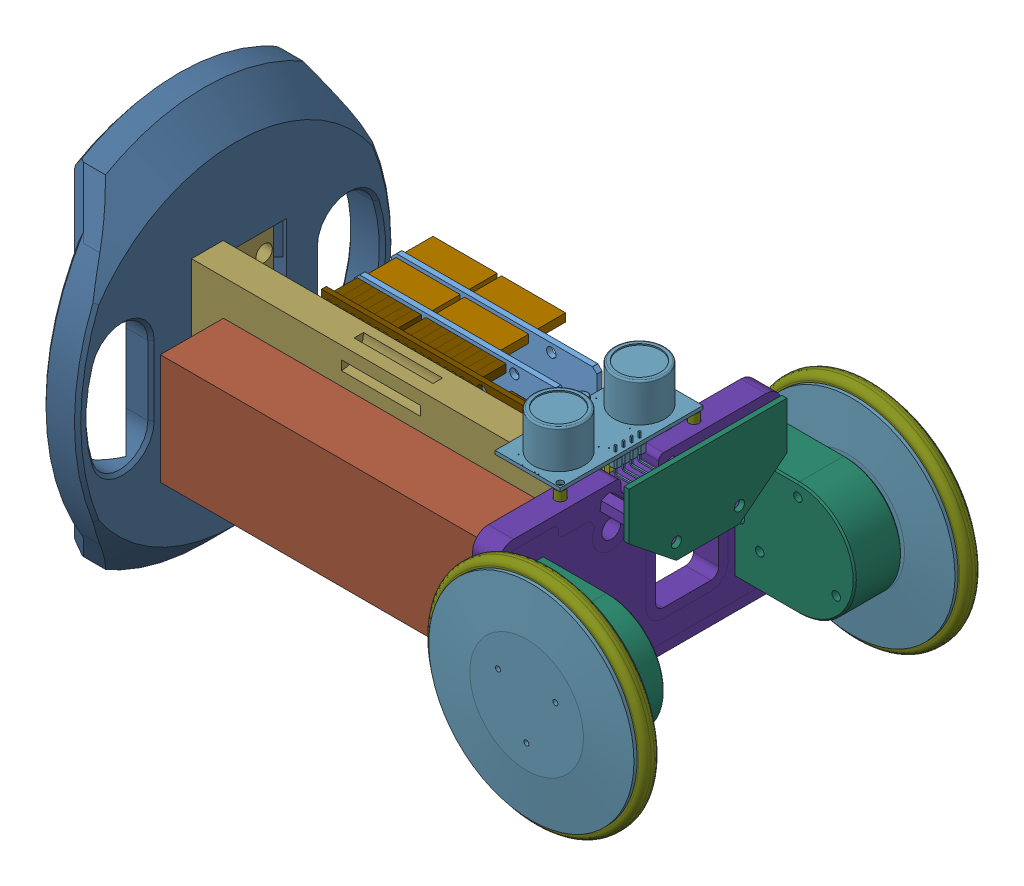
SolidWorks assembly blanceCar-BLDC-双轮平衡平台-立式, configuration 默认. Lengths in mm.
Overall size (212.5 125 111.7).
233 component instances, 36 part files, 54 mates.
Components (placement in the parent):
- BLDC一体驱动-typeA-1: BLDC一体驱动-typeA [默认] at (10.5873 0 95.3779) size (88.95 88.95 25.75)
  - lgt328-simpleFoc-drv8313.step-1: lgt328-simpleFoc-drv8313.step [默认] at origin size (28.6 30.99 10.29)
    - LQFP-32_7x7mm_P0.8mm.step-1: LQFP-32_7x7mm_P0.8mm.step [默认] at (5.381 2.9 1.65) size (9 9 1.5)
      - SOLID.step-1: SOLID.step [默认] at origin size (9 9 1.5)
    - C_0603_1608Metric.step-1: C_0603_1608Metric.step [默认] at (-3.2065 2.01 1.65) x (-1 0 0) z (0 0 1) size (1.6 0.8 0.8)
      - SOLID-0.step-1: SOLID-0.step [默认] at origin size (1.6 0.8 0.8)
    - C_0603_1608Metric.step-2: C_0603_1608Metric.step [默认] at (-3.2165 3.53 1.65) x (-1 0 0) z (0 0 1) size (1.6 0.8 0.8)
      - SOLID-0.step-1: SOLID-0.step [默认] at origin size (1.6 0.8 0.8)
    - C_0603_1608Metric.step-3: C_0603_1608Metric.step [默认] at (0.3835 7.85 1.65) x (-1 0 0) z (0 0 1) size (1.6 0.8 0.8)
      - SOLID-0.step-1: SOLID-0.step [默认] at origin size (1.6 0.8 0.8)
    - SW_SPST_B3U-1000P.step-1: SW_SPST_B3U-1000P.step [默认] at (5.7412 10.211 1.65) size (4 2.51 1.59)
      - SOLID-1.step-1: SOLID-1.step [默认] at origin size (4 2.51 1.59)
    - R_0603_1608Metric.step-1: R_0603_1608Metric.step [默认] at (-9.889 -1.58 1.65) x (0 1 0) z (0 0 1) size (1.6 0.8 0.45)
      - SOLID-2.step-1: SOLID-2.step [默认] at origin size (1.6 0.8 0.45)
    - Resonator_SMD_muRata_CSTxExxV-3Pin_3.0x1.1mm.step-1: Resonator_SMD_muRata_CSTxExxV-3Pin_3.0x1.1mm.step [默认] at (-2.869 6.12 1.65) x (0 -1 0) z (0 0 1) size (3.2 1.35 0.9)
      - SOLID-3.step-1: SOLID-3.step [默认] at origin size (3.2 1.35 0.9)
    - C_0603_1608Metric.step-4: C_0603_1608Metric.step [默认] at (-4.9014 3.2006 -0.05) x (0 1 0) z (0 0 -1) size (1.6 0.8 0.8)
      - SOLID-0.step-1: SOLID-0.step [默认] at origin size (1.6 0.8 0.8)
    - DRV8313PWP.step-1: DRV8313PWP.step [默认] at (-0.019 -8.04 1.65) x (0 1 0) z (1 0 0) size (6.4 1.2 9.7)
      - COMPOUND.step-1: COMPOUND.step [默认] at origin size (6.4 1.2 9.7)
    - PinSocket_1x03_P2.54mm_Vertical.step-1: PinSocket_1x03_P2.54mm_Vertical.step [默认] at (2.541 -13.4 -0.05) x (0 1 0) z (0 0 -1) size (2.54 7.62 10.1)
      - SOLID-4.step-1: SOLID-4.step [默认] at origin size (2.54 7.62 10.1)
    - SOT-89-3.step-1: SOT-89-3.step [默认] at (-6.609 6.85 1.65) x (0 -1 0) z (0 0 1) size (4 4.5 1.52)
      - SOLID-5.step-1: SOLID-5.step [默认] at origin size (4 4.5 1.52)
    - C_0603_1608Metric.step-5: C_0603_1608Metric.step [默认] at (10.251 8.53 1.65) size (1.6 0.8 0.8)
      - SOLID-0.step-1: SOLID-0.step [默认] at origin size (1.6 0.8 0.8)
    - C_0603_1608Metric.step-6: C_0603_1608Metric.step [默认] at (-4.9014 0.2034 -0.05) x (0 1 0) z (0 0 -1) size (1.6 0.8 0.8)
      - SOLID-0.step-1: SOLID-0.step [默认] at origin size (1.6 0.8 0.8)
    - C_0603_1608Metric.step-7: C_0603_1608Metric.step [默认] at (-5.969 -10.4125 1.65) x (0 -1 0) z (0 0 1) size (1.6 0.8 0.8)
      - SOLID-0.step-1: SOLID-0.step [默认] at origin size (1.6 0.8 0.8)
    - C_0603_1608Metric.step-8: C_0603_1608Metric.step [默认] at (-9.889 9.2875 1.65) x (0 1 0) z (0 0 1) size (1.6 0.8 0.8)
      - SOLID-0.step-1: SOLID-0.step [默认] at origin size (1.6 0.8 0.8)
    - C_0603_1608Metric.step-9: C_0603_1608Metric.step [默认] at (7.511 -10.7 1.65) x (0 1 0) z (0 0 1) size (1.6 0.8 0.8)
      - SOLID-0.step-1: SOLID-0.step [默认] at origin size (1.6 0.8 0.8)
    - C_0603_1608Metric.step-10: C_0603_1608Metric.step [默认] at (-3.319 9.4775 1.65) x (0 -1 0) z (0 0 1) size (1.6 0.8 0.8)
      - SOLID-0.step-1: SOLID-0.step [默认] at origin size (1.6 0.8 0.8)
    - C_0603_1608Metric.step-11: C_0603_1608Metric.step [默认] at (6.021 -10.69 1.65) x (0 1 0) z (0 0 1) size (1.6 0.8 0.8)
      - SOLID-0.step-1: SOLID-0.step [默认] at origin size (1.6 0.8 0.8)
    - C_0603_1608Metric.step-12: C_0603_1608Metric.step [默认] at (-5.229 -13.01 1.65) size (1.6 0.8 0.8)
      - SOLID-0.step-1: SOLID-0.step [默认] at origin size (1.6 0.8 0.8)
    - C_0603_1608Metric.step-13: C_0603_1608Metric.step [默认] at (-7.459 -10.4 1.65) x (0 1 0) z (0 0 1) size (1.6 0.8 0.8)
      - SOLID-0.step-1: SOLID-0.step [默认] at origin size (1.6 0.8 0.8)
    - C_0603_1608Metric.step-14: C_0603_1608Metric.step [默认] at (7.531 -7.6825 1.65) x (0 -1 0) z (0 0 1) size (1.6 0.8 0.8)
      - SOLID-0.step-1: SOLID-0.step [默认] at origin size (1.6 0.8 0.8)
    - LED_0603_1608Metric.step-1: LED_0603_1608Metric.step [默认] at (-11.369 6.2825 1.65) x (0 1 0) z (0 0 1) size (1.6 0.8 1.1)
      - SOLID-6.step-1: SOLID-6.step [默认] at origin size (1.6 0.8 1.1)
    - R_0603_1608Metric.step-2: R_0603_1608Metric.step [默认] at (10.611 7.05 1.65) x (-1 0 0) z (0 0 1) size (1.6 0.8 0.45)
      - SOLID-2.step-1: SOLID-2.step [默认] at origin size (1.6 0.8 0.45)
    - R_0603_1608Metric.step-3: R_0603_1608Metric.step [默认] at (-9.869 6.2725 1.65) x (0 -1 0) z (0 0 1) size (1.6 0.8 0.45)
      - SOLID-2.step-1: SOLID-2.step [默认] at origin size (1.6 0.8 0.45)
    - R_0603_1608Metric.step-4: R_0603_1608Metric.step [默认] at (4.931 -1.2425 -0.05) x (0 1 0) z (0 0 -1) size (1.6 0.8 0.45)
      - SOLID-2.step-1: SOLID-2.step [默认] at origin size (1.6 0.8 0.45)
    - R_0603_1608Metric.step-5: R_0603_1608Metric.step [默认] at (2.7186 3.9626 -0.05) x (-1 0 0) z (0 0 -1) size (1.6 0.8 0.45)
      - SOLID-2.step-1: SOLID-2.step [默认] at origin size (1.6 0.8 0.45)
    - R_0603_1608Metric.step-6: R_0603_1608Metric.step [默认] at (4.931 1.7775 -0.05) x (0 -1 0) z (0 0 -1) size (1.6 0.8 0.45)
      - SOLID-2.step-1: SOLID-2.step [默认] at origin size (1.6 0.8 0.45)
    - R_0603_1608Metric.step-7: R_0603_1608Metric.step [默认] at (6.041 -7.6825 1.65) x (0 -1 0) z (0 0 1) size (1.6 0.8 0.45)
      - SOLID-2.step-1: SOLID-2.step [默认] at origin size (1.6 0.8 0.45)
    - SOIC-8-1EP_3.9x4.9mm_P1.27mm_EP2.35x2.35mm.step-1: SOIC-8-1EP_3.9x4.9mm_P1.27mm_EP2.35x2.35mm.step [默认] at (0.001 0 -0.05) x (1 0 0) z (0 0 -1) size (6 4.9 1.75)
      - SOLID-7.step-1: SOLID-7.step [默认] at origin size (6 4.9 1.75)
    - COMPOUND-8.step-1: COMPOUND-8.step [默认] at origin size (28.6 30.99 1.6)
  - 零件2^BLDC一体驱动-typeA-1: 零件2^BLDC一体驱动-typeA [默认] at (0.001 0 -17.8) x (0.869437 -0.494044 0) z (-0.494044 -0.869437 0) size (32 15 32) (virtual)
  - 零件3^BLDC一体驱动-typeA-1: 零件3^BLDC一体驱动-typeA [默认] at (0.001 0 -4.8) x (0.869437 -0.494044 0) z (0 0 1) size (26.77 30.2 4.8) (virtual)
  - 零件4^BLDC一体驱动-typeA-1: 零件4^BLDC一体驱动-typeA [默认] at (0.001 0 -14.3) x (0.862573 0.505933 0) z (0 0 1) size (65 65 10) (virtual)
  - 零件5^BLDC一体驱动-typeA-1: 零件5^BLDC一体驱动-typeA [默认] at (0.001 0 -1.05) x (0.000169 -1 0) z (0 0 -1) size (36 38 15) (virtual)
  - 零件1^BLDC一体驱动-typeA-1: 零件1^BLDC一体驱动-typeA [默认] at (0.001 0 -14.3) x (1 0 0) z (0 1 0) size (70 5 70) (virtual)
- BLDC一体驱动-typeA-2: BLDC一体驱动-typeA [默认] at (10.5873 0 168.4779) x (1 0.000338 0) z (0 0 -1) size (88.95 88.95 25.75)
  - lgt328-simpleFoc-drv8313.step-1: lgt328-simpleFoc-drv8313.step [默认] at origin size (28.6 30.99 10.29)
    - LQFP-32_7x7mm_P0.8mm.step-1: LQFP-32_7x7mm_P0.8mm.step [默认] at (5.381 2.9 1.65) size (9 9 1.5)
      - SOLID.step-1: SOLID.step [默认] at origin size (9 9 1.5)
    - C_0603_1608Metric.step-1: C_0603_1608Metric.step [默认] at (-3.2065 2.01 1.65) x (-1 0 0) z (0 0 1) size (1.6 0.8 0.8)
      - SOLID-0.step-1: SOLID-0.step [默认] at origin size (1.6 0.8 0.8)
    - C_0603_1608Metric.step-2: C_0603_1608Metric.step [默认] at (-3.2165 3.53 1.65) x (-1 0 0) z (0 0 1) size (1.6 0.8 0.8)
      - SOLID-0.step-1: SOLID-0.step [默认] at origin size (1.6 0.8 0.8)
    - C_0603_1608Metric.step-3: C_0603_1608Metric.step [默认] at (0.3835 7.85 1.65) x (-1 0 0) z (0 0 1) size (1.6 0.8 0.8)
      - SOLID-0.step-1: SOLID-0.step [默认] at origin size (1.6 0.8 0.8)
    - SW_SPST_B3U-1000P.step-1: SW_SPST_B3U-1000P.step [默认] at (5.7412 10.211 1.65) size (4 2.51 1.59)
      - SOLID-1.step-1: SOLID-1.step [默认] at origin size (4 2.51 1.59)
    - R_0603_1608Metric.step-1: R_0603_1608Metric.step [默认] at (-9.889 -1.58 1.65) x (0 1 0) z (0 0 1) size (1.6 0.8 0.45)
      - SOLID-2.step-1: SOLID-2.step [默认] at origin size (1.6 0.8 0.45)
    - Resonator_SMD_muRata_CSTxExxV-3Pin_3.0x1.1mm.step-1: Resonator_SMD_muRata_CSTxExxV-3Pin_3.0x1.1mm.step [默认] at (-2.869 6.12 1.65) x (0 -1 0) z (0 0 1) size (3.2 1.35 0.9)
      - SOLID-3.step-1: SOLID-3.step [默认] at origin size (3.2 1.35 0.9)
    - C_0603_1608Metric.step-4: C_0603_1608Metric.step [默认] at (-4.9014 3.2006 -0.05) x (0 1 0) z (0 0 -1) size (1.6 0.8 0.8)
      - SOLID-0.step-1: SOLID-0.step [默认] at origin size (1.6 0.8 0.8)
    - DRV8313PWP.step-1: DRV8313PWP.step [默认] at (-0.019 -8.04 1.65) x (0 1 0) z (1 0 0) size (6.4 1.2 9.7)
      - COMPOUND.step-1: COMPOUND.step [默认] at origin size (6.4 1.2 9.7)
    - PinSocket_1x03_P2.54mm_Vertical.step-1: PinSocket_1x03_P2.54mm_Vertical.step [默认] at (2.541 -13.4 -0.05) x (0 1 0) z (0 0 -1) size (2.54 7.62 10.1)
      - SOLID-4.step-1: SOLID-4.step [默认] at origin size (2.54 7.62 10.1)
    - SOT-89-3.step-1: SOT-89-3.step [默认] at (-6.609 6.85 1.65) x (0 -1 0) z (0 0 1) size (4 4.5 1.52)
      - SOLID-5.step-1: SOLID-5.step [默认] at origin size (4 4.5 1.52)
    - C_0603_1608Metric.step-5: C_0603_1608Metric.step [默认] at (10.251 8.53 1.65) size (1.6 0.8 0.8)
      - SOLID-0.step-1: SOLID-0.step [默认] at origin size (1.6 0.8 0.8)
    - C_0603_1608Metric.step-6: C_0603_1608Metric.step [默认] at (-4.9014 0.2034 -0.05) x (0 1 0) z (0 0 -1) size (1.6 0.8 0.8)
      - SOLID-0.step-1: SOLID-0.step [默认] at origin size (1.6 0.8 0.8)
    - C_0603_1608Metric.step-7: C_0603_1608Metric.step [默认] at (-5.969 -10.4125 1.65) x (0 -1 0) z (0 0 1) size (1.6 0.8 0.8)
      - SOLID-0.step-1: SOLID-0.step [默认] at origin size (1.6 0.8 0.8)
    - C_0603_1608Metric.step-8: C_0603_1608Metric.step [默认] at (-9.889 9.2875 1.65) x (0 1 0) z (0 0 1) size (1.6 0.8 0.8)
      - SOLID-0.step-1: SOLID-0.step [默认] at origin size (1.6 0.8 0.8)
    - C_0603_1608Metric.step-9: C_0603_1608Metric.step [默认] at (7.511 -10.7 1.65) x (0 1 0) z (0 0 1) size (1.6 0.8 0.8)
      - SOLID-0.step-1: SOLID-0.step [默认] at origin size (1.6 0.8 0.8)
    - C_0603_1608Metric.step-10: C_0603_1608Metric.step [默认] at (-3.319 9.4775 1.65) x (0 -1 0) z (0 0 1) size (1.6 0.8 0.8)
      - SOLID-0.step-1: SOLID-0.step [默认] at origin size (1.6 0.8 0.8)
    - C_0603_1608Metric.step-11: C_0603_1608Metric.step [默认] at (6.021 -10.69 1.65) x (0 1 0) z (0 0 1) size (1.6 0.8 0.8)
      - SOLID-0.step-1: SOLID-0.step [默认] at origin size (1.6 0.8 0.8)
    - C_0603_1608Metric.step-12: C_0603_1608Metric.step [默认] at (-5.229 -13.01 1.65) size (1.6 0.8 0.8)
      - SOLID-0.step-1: SOLID-0.step [默认] at origin size (1.6 0.8 0.8)
    - C_0603_1608Metric.step-13: C_0603_1608Metric.step [默认] at (-7.459 -10.4 1.65) x (0 1 0) z (0 0 1) size (1.6 0.8 0.8)
      - SOLID-0.step-1: SOLID-0.step [默认] at origin size (1.6 0.8 0.8)
    - C_0603_1608Metric.step-14: C_0603_1608Metric.step [默认] at (7.531 -7.6825 1.65) x (0 -1 0) z (0 0 1) size (1.6 0.8 0.8)
      - SOLID-0.step-1: SOLID-0.step [默认] at origin size (1.6 0.8 0.8)
    - LED_0603_1608Metric.step-1: LED_0603_1608Metric.step [默认] at (-11.369 6.2825 1.65) x (0 1 0) z (0 0 1) size (1.6 0.8 1.1)
      - SOLID-6.step-1: SOLID-6.step [默认] at origin size (1.6 0.8 1.1)
    - R_0603_1608Metric.step-2: R_0603_1608Metric.step [默认] at (10.611 7.05 1.65) x (-1 0 0) z (0 0 1) size (1.6 0.8 0.45)
      - SOLID-2.step-1: SOLID-2.step [默认] at origin size (1.6 0.8 0.45)
    - R_0603_1608Metric.step-3: R_0603_1608Metric.step [默认] at (-9.869 6.2725 1.65) x (0 -1 0) z (0 0 1) size (1.6 0.8 0.45)
      - SOLID-2.step-1: SOLID-2.step [默认] at origin size (1.6 0.8 0.45)
    - R_0603_1608Metric.step-4: R_0603_1608Metric.step [默认] at (4.931 -1.2425 -0.05) x (0 1 0) z (0 0 -1) size (1.6 0.8 0.45)
      - SOLID-2.step-1: SOLID-2.step [默认] at origin size (1.6 0.8 0.45)
    - R_0603_1608Metric.step-5: R_0603_1608Metric.step [默认] at (2.7186 3.9626 -0.05) x (-1 0 0) z (0 0 -1) size (1.6 0.8 0.45)
      - SOLID-2.step-1: SOLID-2.step [默认] at origin size (1.6 0.8 0.45)
    - R_0603_1608Metric.step-6: R_0603_1608Metric.step [默认] at (4.931 1.7775 -0.05) x (0 -1 0) z (0 0 -1) size (1.6 0.8 0.45)
      - SOLID-2.step-1: SOLID-2.step [默认] at origin size (1.6 0.8 0.45)
    - R_0603_1608Metric.step-7: R_0603_1608Metric.step [默认] at (6.041 -7.6825 1.65) x (0 -1 0) z (0 0 1) size (1.6 0.8 0.45)
      - SOLID-2.step-1: SOLID-2.step [默认] at origin size (1.6 0.8 0.45)
    - SOIC-8-1EP_3.9x4.9mm_P1.27mm_EP2.35x2.35mm.step-1: SOIC-8-1EP_3.9x4.9mm_P1.27mm_EP2.35x2.35mm.step [默认] at (0.001 0 -0.05) x (1 0 0) z (0 0 -1) size (6 4.9 1.75)
      - SOLID-7.step-1: SOLID-7.step [默认] at origin size (6 4.9 1.75)
    - COMPOUND-8.step-1: COMPOUND-8.step [默认] at origin size (28.6 30.99 1.6)
  - 零件2^BLDC一体驱动-typeA-1: 零件2^BLDC一体驱动-typeA [默认] at (0.001 0 -17.8) x (0.869437 -0.494044 0) z (-0.494044 -0.869437 0) size (32 15 32) (virtual)
  - 零件3^BLDC一体驱动-typeA-1: 零件3^BLDC一体驱动-typeA [默认] at (0.001 0 -4.8) x (0.869437 -0.494044 0) z (0 0 1) size (26.77 30.2 4.8) (virtual)
  - 零件4^BLDC一体驱动-typeA-1: 零件4^BLDC一体驱动-typeA [默认] at (0.001 0 -14.3) x (0.862573 0.505933 0) z (0 0 1) size (65 65 10) (virtual)
  - 零件5^BLDC一体驱动-typeA-1: 零件5^BLDC一体驱动-typeA [默认] at (0.001 0 -1.05) x (0.000169 -1 0) z (0 0 -1) size (36 38 15) (virtual)
  - 零件1^BLDC一体驱动-typeA-1: 零件1^BLDC一体驱动-typeA [默认] at (0.001 0 -14.3) x (1 0 0) z (0 1 0) size (70 5 70) (virtual)
- 零件8^blanceCar-BLDC-双轮平衡平台-立式-1: 零件8^blanceCar-BLDC-双轮平衡平台-立式 [默认] at (-13.4117 -0.0041 94.4279) x (0.000169 -1 0) z (-1 -0.000169 0) size (55 90 8)
- ESP32-WROOM-32 AZ-Delivery-1: ESP32-WROOM-32 AZ-Delivery [默认] at (-77.5199 0.0218 131.3779) x (-1 -0.000169 0) z (0 0 -1) size (70.33 53.34 15.2)
- ArduinoFOC-1: ArduinoFOC [Default] at (-43.1784 -26.5154 121.1864) x (-1 -0.000169 0) z (0 0 -1) size (68.73 53.73 23.8)
  - Board-1: Board [Default] at origin size (68.05 53.25 1.7)
  - CAP1-1: CAP1 [Default] at origin size (7.3 6.6 7.7)
    - User_Library-A3D-003-00012-1: User_Library-A3D-003-00012 [Default] at (37.9 15.65 0) x (1 0 0) z (0 0 1) size (7.3 6.6 7.7)
  - R1-1: R1 [Default] at origin size (3.35 2.64 0.9)
    - 5920132160-1: 5920132160 [Default] at (12 10 0) size (3.35 2.64 0.9)
      - Extruded-1: Extruded [Default] at origin size (3.35 2.64 0.9)
  - PULL_I-1: PULL_I [Default] at origin size (3.35 2.64 0.9)
    - 5920132160-1: 5920132160 [Default] at (46.25 33.75 0) size (3.35 2.64 0.9)
      - Extruded-1: Extruded [Default] at origin size (3.35 2.64 0.9)
  - R2-1: R2 [Default] at origin size (3.35 2.64 0.9)
    - 5920132160-1: 5920132160 [Default] at (37.5 44.25 0) size (3.35 2.64 0.9)
      - Extruded-1: Extruded [Default] at origin size (3.35 2.64 0.9)
  - PULL_A-1: PULL_A [Default] at origin size (3.35 2.64 0.9)
    - 5920132160-1: 5920132160 [Default] at (46.277 43.877 0) size (3.35 2.64 0.9)
      - Extruded-1: Extruded [Default] at origin size (3.35 2.64 0.9)
  - PULL_B-1: PULL_B [Default] at origin size (3.35 2.64 0.9)
    - 5920132160-1: 5920132160 [Default] at (46.25 38.75 0) size (3.35 2.64 0.9)
      - Extruded-1: Extruded [Default] at origin size (3.35 2.64 0.9)
  - L6234-1: L6234 [Default] at origin size (16.01 14.5 3.85)
    - L6234PD-1: L6234PD [Default] at (20.7048 33.6248 0.2) x (1 0 0) z (0 -1 0) size (16 3.65 14.5)
    - L6234PD-2: L6234PD [Default] at (20.6947 33.6248 0) x (1 0 0) z (0 -1 0) size (16 3.65 14.5)
  - BAT1-1: BAT1 [Default] at origin size (2.92 2.34 1)
    - User_Library-BAT54-1: User_Library-BAT54 [Default] at (34.9999 26.7499 0) x (1 0 0) z (0 0 1) size (2.92 2.34 1)
    - User_Library-BAT54-2: User_Library-BAT54 [Default] at (35 26.7499 0) x (1 0 0) z (0 0 1) size (2.92 2.34 1)
  - TB_PWR-1: TB_PWR [Default] at origin size (10 9 17.6)
    - 2_RGB15238730-1: 2_RGB15238730 [Default] at (36.3474 54.5994 -15.5) x (0 -1 0) z (-1 0 0) size (9 17.6 10)
  - TB_M1-1: TB_M1 [Default] at origin size (9.8 15.74 17.3)
    - 37753_RGB15238730-1: 37753_RGB15238730 [Default] at (0.4361 31.1706 0) x (-1 0 0) z (0 1 0) size (9.8 17.3 15.74)
  - C4-1: C4 [Default] at origin size (1.8 3.4 1.3)
    - 5920131968-1: 5920131968 [Default] at (17 42.5 0) size (1.8 3.4 1.3)
      - Extruded_2-1: Extruded_2 [Default] at origin size (1.8 3.4 1.3)
  - C3-1: C3 [Default] at origin size (1.8 3.4 1.3)
    - 5920131968-1: 5920131968 [Default] at (20.5 42.5 0) size (1.8 3.4 1.3)
      - Extruded_2-1: Extruded_2 [Default] at origin size (1.8 3.4 1.3)
  - C2-1: C2 [Default] at origin size (1.8 3.4 1.3)
    - 5920131968-1: 5920131968 [Default] at (35 32.25 0) size (1.8 3.4 1.3)
      - Extruded_2-1: Extruded_2 [Default] at origin size (1.8 3.4 1.3)
  - C1-1: C1 [Default] at origin size (1.8 3.4 1.3)
    - 5920131968-1: 5920131968 [Default] at (32.5 40.75 0) size (1.8 3.4 1.3)
      - Extruded_2-1: Extruded_2 [Default] at origin size (1.8 3.4 1.3)
  - headers-1: headers [Default] at (0.4047 0.2078 0) size (42.02 50.5 20)
- ArduinoFOC-2: ArduinoFOC [Default] at (-43.1784 -26.5154 109.495) x (-1 -0.000169 0) z (0 0 -1) size (68.73 53.73 23.8)
  - Board-1: Board [Default] at origin size (68.05 53.25 1.7)
  - CAP1-1: CAP1 [Default] at origin size (7.3 6.6 7.7)
    - User_Library-A3D-003-00012-1: User_Library-A3D-003-00012 [Default] at (37.9 15.65 0) x (1 0 0) z (0 0 1) size (7.3 6.6 7.7)
  - R1-1: R1 [Default] at origin size (3.35 2.64 0.9)
    - 5920132160-1: 5920132160 [Default] at (12 10 0) size (3.35 2.64 0.9)
      - Extruded-1: Extruded [Default] at origin size (3.35 2.64 0.9)
  - PULL_I-1: PULL_I [Default] at origin size (3.35 2.64 0.9)
    - 5920132160-1: 5920132160 [Default] at (46.25 33.75 0) size (3.35 2.64 0.9)
      - Extruded-1: Extruded [Default] at origin size (3.35 2.64 0.9)
  - R2-1: R2 [Default] at origin size (3.35 2.64 0.9)
    - 5920132160-1: 5920132160 [Default] at (37.5 44.25 0) size (3.35 2.64 0.9)
      - Extruded-1: Extruded [Default] at origin size (3.35 2.64 0.9)
  - PULL_A-1: PULL_A [Default] at origin size (3.35 2.64 0.9)
    - 5920132160-1: 5920132160 [Default] at (46.277 43.877 0) size (3.35 2.64 0.9)
      - Extruded-1: Extruded [Default] at origin size (3.35 2.64 0.9)
  - PULL_B-1: PULL_B [Default] at origin size (3.35 2.64 0.9)
    - 5920132160-1: 5920132160 [Default] at (46.25 38.75 0) size (3.35 2.64 0.9)
      - Extruded-1: Extruded [Default] at origin size (3.35 2.64 0.9)
  - L6234-1: L6234 [Default] at origin size (16.01 14.5 3.85)
    - L6234PD-1: L6234PD [Default] at (20.7048 33.6248 0.2) x (1 0 0) z (0 -1 0) size (16 3.65 14.5)
    - L6234PD-2: L6234PD [Default] at (20.6947 33.6248 0) x (1 0 0) z (0 -1 0) size (16 3.65 14.5)
  - BAT1-1: BAT1 [Default] at origin size (2.92 2.34 1)
    - User_Library-BAT54-1: User_Library-BAT54 [Default] at (34.9999 26.7499 0) x (1 0 0) z (0 0 1) size (2.92 2.34 1)
    - User_Library-BAT54-2: User_Library-BAT54 [Default] at (35 26.7499 0) x (1 0 0) z (0 0 1) size (2.92 2.34 1)
  - TB_PWR-1: TB_PWR [Default] at origin size (10 9 17.6)
    - 2_RGB15238730-1: 2_RGB15238730 [Default] at (36.3474 54.5994 -15.5) x (0 -1 0) z (-1 0 0) size (9 17.6 10)
  - TB_M1-1: TB_M1 [Default] at origin size (9.8 15.74 17.3)
    - 37753_RGB15238730-1: 37753_RGB15238730 [Default] at (0.4361 31.1706 0) x (-1 0 0) z (0 1 0) size (9.8 17.3 15.74)
  - C4-1: C4 [Default] at origin size (1.8 3.4 1.3)
    - 5920131968-1: 5920131968 [Default] at (17 42.5 0) size (1.8 3.4 1.3)
      - Extruded_2-1: Extruded_2 [Default] at origin size (1.8 3.4 1.3)
  - C3-1: C3 [Default] at origin size (1.8 3.4 1.3)
    - 5920131968-1: 5920131968 [Default] at (20.5 42.5 0) size (1.8 3.4 1.3)
      - Extruded_2-1: Extruded_2 [Default] at origin size (1.8 3.4 1.3)
  - C2-1: C2 [Default] at origin size (1.8 3.4 1.3)
    - 5920131968-1: 5920131968 [Default] at (35 32.25 0) size (1.8 3.4 1.3)
      - Extruded_2-1: Extruded_2 [Default] at origin size (1.8 3.4 1.3)
  - C1-1: C1 [Default] at origin size (1.8 3.4 1.3)
    - 5920131968-1: 5920131968 [Default] at (32.5 40.75 0) size (1.8 3.4 1.3)
      - Extruded_2-1: Extruded_2 [Default] at origin size (1.8 3.4 1.3)
  - headers-1: headers [Default] at (0.4047 0.2078 0) size (42.02 50.5 20)
- top_plate-1: top_plate [Default] at (-142.4117 -0.0259 131.9279) x (0.000169 -1 0) z (0 0 -1) size (125 20 100.25)
- battery3-1: battery3 [Default] at (-80.1656 -0.2982 145.9279) x (1 0.000169 0) z (0.000169 -1 0) size (105 20 35)
- 零件1^blanceCar-BLDC-双轮平衡平台-立式-1: 零件1^blanceCar-BLDC-双轮平衡平台-立式 [默认] at (-77.4117 -0.0149 140.9279) x (0 0 1) z (1 0.000169 0) size (26 55 125.25) (virtual)
- mpu6050-1: mpu6050 [Default] at (-143.6114 -2.059 132.6308) x (-0.000169 1 0) z (0 0 -1) size (21.2 14 16)
- hc-sr04-1: hc-sr04 [Detailed] at (-22.3169 30.4944 131.9279) x (0 0 -1) z (1 0.000169 0) size (45.2 18.55 25.75)
- 零件2^blanceCar-BLDC-双轮平衡平台-立式-1: 零件2^blanceCar-BLDC-双轮平衡平台-立式 [默认] at (12.182 37.0003 131.9279) x (0 0 -1) z (-0.000169 1 0) size (50 1.6 27) (virtual)
- 零件3^blanceCar-BLDC-双轮平衡平台-立式-1: 零件3^blanceCar-BLDC-双轮平衡平台-立式 [默认] at (-13.4157 23.4959 110.7279) x (1 0.000169 0) z (0 0 1) size (3 7 3) (virtual)
- 零件3^blanceCar-BLDC-双轮平衡平台-立式-2: 零件3^blanceCar-BLDC-双轮平衡平台-立式 [默认] at (-48.007 23.1828 29.2495) size (3 7 3) (hidden, virtual)
- 零件3^blanceCar-BLDC-双轮平衡平台-立式-3: 零件3^blanceCar-BLDC-双轮平衡平台-立式 [默认] at (-13.4157 23.4959 153.1279) x (1 0.000169 0) z (0 0 1) size (3 7 3) (virtual)
- 零件4^blanceCar-BLDC-双轮平衡平台-立式-3: 零件4^blanceCar-BLDC-双轮平衡平台-立式 [默认] at (10.5845 22.5 141.9279) x (0.000065 -0.382574 0.923925) z (0.000156 -0.923925 -0.382574) size (5.54 20 4.8) (virtual)
- 零件4^blanceCar-BLDC-双轮平衡平台-立式-4: 零件4^blanceCar-BLDC-双轮平衡平台-立式 [默认] at (10.5845 22.5 121.9279) x (0.000065 -0.382574 0.923925) z (0.000156 -0.923925 -0.382574) size (5.54 20 4.8) (virtual)
- 零件5^blanceCar-BLDC-双轮平衡平台-立式-1: 零件5^blanceCar-BLDC-双轮平衡平台-立式 [默认] at (-57.1958 -24.1048 141.9279) x (1 0 0) z (0 1 0) size (5.36 9 5.35) (virtual)
- 零件5^blanceCar-BLDC-双轮平衡平台-立式-2: 零件5^blanceCar-BLDC-双轮平衡平台-立式 [默认] at (-109.2714 8.9064 141.9279) x (1 0 0) z (0 1 0) size (5.36 9 5.35) (virtual)
- 零件5^blanceCar-BLDC-双轮平衡平台-立式-3: 零件5^blanceCar-BLDC-双轮平衡平台-立式 [默认] at (-109.2667 -19.0336 141.9279) x (1 0 0) z (0 1 0) size (5.36 9 5.35) (virtual)
- 零件5^blanceCar-BLDC-双轮平衡平台-立式-4: 零件5^blanceCar-BLDC-双轮平衡平台-立式 [默认] at (-58.4735 24.1383 141.9279) x (0.967415 -0.253196 0) z (0.253196 0.967415 0) size (5.36 9 5.35) (virtual)
Mates (geometry in assembly coordinates):
- 重合1: coincident aligned: plane of BLDC一体驱动-typeA-1/零件5^BLDC一体驱动-typeA-1 through (-9.4117 -0.0034 86.8279) normal (-1 -0.000169 0); plane of BLDC一体驱动-typeA-2/零件5^BLDC一体驱动-typeA-1 through (-9.4117 -0.0034 177.0279) normal (-1 -0.000169 0)
- 重合2: coincident aligned: plane of BLDC一体驱动-typeA-1/零件5^BLDC一体驱动-typeA-1 through (10.5852 18 86.8279) normal (-0.000169 1 0); plane of BLDC一体驱动-typeA-2/零件5^BLDC一体驱动-typeA-1 through (10.5852 18 177.0279) normal (-0.000169 1 0)
- 同心1: concentric aligned: cylinder of 零件8^blanceCar-BLDC-双轮平衡平台-立式-1 through (-7.4134 9.997 169.5279) axis (-1 -0.000169 0) radius 1.6; circle of BLDC一体驱动-typeA-2/零件5^BLDC一体驱动-typeA-1
- 重合3: coincident anti-aligned: plane of ArduinoFOC-1/headers-1 through (-43.5831 -26.3077 111.1864) normal (0 0 -1); plane of ArduinoFOC-2/Board-1 through (-43.9636 -25.4805 111.1864) normal (0 0 1)
- 同心2: concentric anti-aligned: cylinder of ArduinoFOC-1/headers-1 through (-106.0836 -23.7782 111.1864) axis (0 0 1) radius 0.5; cylinder of ArduinoFOC-2/headers-1 through (-106.0836 -23.7782 119.495) axis (0 0 -1) radius 0.5
- 重合4: coincident anti-aligned: plane of ESP32-WROOM-32 AZ-Delivery-1 through (-95.552 -25.3957 122.8779) normal (0 0 -1); plane of ArduinoFOC-1/Board-1 through (-43.9636 -25.4805 122.8779) normal (0 0 1)
- 重合5: coincident aligned: plane of ESP32-WROOM-32 AZ-Delivery-1 through (-111.8063 -21.574 132.9279) normal (-1 -0.000169 0); plane of ArduinoFOC-1/Board-1 through (-111.8063 -21.527 122.8779) normal (-1 -0.000169 0)
- 重合6: coincident aligned: plane of ESP32-WROOM-32 AZ-Delivery-1 through (-43.2254 -26.6424 132.9279) normal (0.000169 -1 0); plane of ArduinoFOC-1/Board-1 through (-45.1784 -26.6427 122.8779) normal (0.000169 -1 0)
- 平行1: parallel aligned: plane of ESP32-WROOM-32 AZ-Delivery-1 through (-60.061 24.1381 132.9279) normal (0 0 1); plane of 零件8^blanceCar-BLDC-双轮平衡平台-立式-1 through (-17.4164 27.4953 176.9279) normal (0 0 1)
- 重合8: coincident aligned: plane of ArduinoFOC-1/Board-1 through (-107.1874 26.6008 122.8779) normal (-0.000169 1 0); plane of ArduinoFOC-2/Board-1 through (-107.1874 26.6008 111.1864) normal (-0.000169 1 0)
- 平行2: parallel anti-aligned: plane of 零件8^blanceCar-BLDC-双轮平衡平台-立式-1 through (-17.4117 -0.0047 94.4279) normal (-1 -0.000169 0); plane of ESP32-WROOM-32 AZ-Delivery-1 through (-43.2344 26.6976 132.9279) normal (1 0.000169 0)
- 平行3: parallel anti-aligned: plane of 零件8^blanceCar-BLDC-双轮平衡平台-立式-1 through (-17.4117 -0.0047 94.4279) normal (-1 -0.000169 0); plane of top_plate-1 through (-137.4117 -0.025 131.9279) normal (1 0.000169 0)
- 平行4: parallel aligned: plane of 零件8^blanceCar-BLDC-双轮平衡平台-立式-1 through (-9.4117 -0.0034 94.4279) normal (1 0.000169 0); plane of battery3-1 through (-22.3112 16.2116 165.9279) normal (1 0.000169 0)
- 平行5: parallel aligned: plane of 零件8^blanceCar-BLDC-双轮平衡平台-立式-1 through (-17.4071 -27.5047 176.9279) normal (0.000169 -1 0); plane of battery3-1 through (-127.3053 -18.8062 165.9279) normal (0.000169 -1 0)
- 重合13: coincident anti-aligned: plane of 零件8^blanceCar-BLDC-双轮平衡平台-立式-1 through (-17.4117 -0.0047 94.4279) normal (-1 -0.000169 0); plane of 零件1^blanceCar-BLDC-双轮平衡平台-立式-1 through (-17.4071 -27.5047 135.9279) normal (1 0.000169 0)
- 重合14: coincident aligned: plane of 零件8^blanceCar-BLDC-双轮平衡平台-立式-1 through (-17.4071 -27.5047 176.9279) normal (0.000169 -1 0); plane of 零件1^blanceCar-BLDC-双轮平衡平台-立式-1 through (-77.4071 -27.5149 140.9279) normal (0.000169 -1 0)
- 重合15: coincident anti-aligned: plane of battery3-1 through (-80.1656 -0.2982 145.9279) normal (0 0 -1); plane of 零件1^blanceCar-BLDC-双轮平衡平台-立式-1 through (-137.4071 -27.525 145.9279) normal (0 0 1)
- 同心3: concentric aligned: cylinder of ESP32-WROOM-32 AZ-Delivery-1 through (-109.2085 -19.0702 132.9279) axis (0 0 -1) radius 1.5875; cylinder of 零件1^blanceCar-BLDC-双轮平衡平台-立式-1 through (-109.2085 -19.0702 140.9279) axis (0 0 -1) radius 2.5
- 距离3: distance = 3 mm anti-aligned: plane of ESP32-WROOM-32 AZ-Delivery-1 through (-60.061 24.1381 132.9279) normal (0 0 1); plane of 零件1^blanceCar-BLDC-双轮平衡平台-立式-1 through (-137.4071 -27.525 135.9279) normal (0 0 -1)
- 同心4: concentric aligned: cylinder of 零件8^blanceCar-BLDC-双轮平衡平台-立式-1 through (-19.4143 14.9949 140.9279) axis (1 0.000169 0) radius 1.6; cylinder of 零件1^blanceCar-BLDC-双轮平衡平台-立式-1 through (-25.4143 14.9939 140.9279) axis (1 0.000169 0) radius 2.6
- 重合31: coincident anti-aligned: plane of top_plate-1 through (-137.4078 -23.525 131.9279) normal (-0.000169 1 0); plane of 零件1^blanceCar-BLDC-双轮平衡平台-立式-1 through (-142.4078 -23.5259 119.9279) normal (0.000169 -1 0)
- 重合32: coincident anti-aligned: plane of top_plate-1 through (-142.4117 -0.0259 131.9279) normal (1 0.000169 0); plane of 零件1^blanceCar-BLDC-双轮平衡平台-立式-1 through (-142.4117 -0.0259 140.9279) normal (-1 -0.000169 0)
- 重合36: coincident anti-aligned: plane of top_plate-1 through (-137.4117 -0.025 145.9279) normal (0 0 -1); plane of 零件1^blanceCar-BLDC-双轮平衡平台-立式-1 through (-137.4071 -27.525 145.9279) normal (0 0 1)
- 重合37: coincident anti-aligned: plane of 零件1^blanceCar-BLDC-双轮平衡平台-立式-1 through (-138.4099 -10.5252 123.1779) normal (0 0 1); plane of mpu6050-1 through (-138.4099 -10.7252 123.1779) normal (0 0 -1)
- 距离1: distance = 4 mm aligned: plane of 零件1^blanceCar-BLDC-双轮平衡平台-立式-1 through (-137.4117 -0.025 140.9279) normal (1 0.000169 0); plane of mpu6050-1 through (-141.4114 -2.0586 132.6308) normal (1 0.000169 0)
- 同心5: concentric aligned: cylinder of 零件8^blanceCar-BLDC-双轮平衡平台-立式-1 through (-13.4157 23.4959 153.1279) axis (-0.000169 1 0) radius 1.6; cylinder of hc-sr04-1 through (-13.416 25.1459 153.1279) axis (-0.000169 1 0) radius 1
- 距离4: distance = 3 mm anti-aligned: plane of 零件8^blanceCar-BLDC-双轮平衡平台-立式-1 through (-17.4164 27.4953 176.9279) normal (-0.000169 1 0); plane of hc-sr04-1 through (-22.3169 30.4944 131.9279) normal (0.000169 -1 0)
- 平行11: parallel aligned: plane of 零件8^blanceCar-BLDC-双轮平衡平台-立式-1 through (-9.4117 -0.0034 94.4279) normal (1 0.000169 0); plane of hc-sr04-1 through (-12.0171 31.5962 109.3279) normal (1 0.000169 0)
- 同心6: concentric aligned: cylinder of 零件8^blanceCar-BLDC-双轮平衡平台-立式-1 through (-17.4155 22.4953 141.9279) axis (1 0.000169 0) radius 2.5; cylinder of 零件2^blanceCar-BLDC-双轮平衡平台-立式-1 through (0.5845 22.4983 141.9279) axis (1 0.000169 0) radius 1.6
- 平行12: parallel aligned: plane of 零件8^blanceCar-BLDC-双轮平衡平台-立式-1 through (-17.4164 27.4953 176.9279) normal (-0.000169 1 0); plane of 零件2^blanceCar-BLDC-双轮平衡平台-立式-1 through (10.5808 44.5 156.9279) normal (-0.000169 1 0)
- 重合47: coincident anti-aligned: plane of BLDC一体驱动-typeA-1/零件5^BLDC一体驱动-typeA-1 through (-9.4117 -0.0034 86.8279) normal (-1 -0.000169 0); plane of 零件8^blanceCar-BLDC-双轮平衡平台-立式-1 through (-9.4117 -0.0034 94.4279) normal (1 0.000169 0)
- 同心7: concentric aligned: cylinder of BLDC一体驱动-typeA-1/零件5^BLDC一体驱动-typeA-1 through (-4.4134 9.9975 94.3279) axis (-1 -0.000169 0) radius 2.6; cylinder of 零件8^blanceCar-BLDC-双轮平衡平台-立式-1 through (-7.4134 9.997 94.3279) axis (-1 -0.000169 0) radius 1.6
- 同心8: concentric aligned: cylinder of 零件8^blanceCar-BLDC-双轮平衡平台-立式-1 through (-7.41 -10.003 94.3279) axis (-1 -0.000169 0) radius 1.6; circle of BLDC一体驱动-typeA-1/零件5^BLDC一体驱动-typeA-1
- 重合48: coincident: line of 零件1^blanceCar-BLDC-双轮平衡平台-立式-1 through (-142.4135 10.4741 139.1779) axis (0 0 -1); plane of mpu6050-1 through (-141.4135 10.4743 139.1779) normal (-0.000169 1 0)
- 同心9: concentric anti-aligned: cylinder of 零件8^blanceCar-BLDC-双轮平衡平台-立式-1 through (-13.4157 23.4959 110.7279) axis (-0.000169 1 0) radius 1.6; cylinder of 铜柱M2*7-1 through (-13.4169 30.4959 110.7279) axis (0.000169 -1 0) radius 1.5
- 同心10: concentric anti-aligned: cylinder of 零件8^blanceCar-BLDC-双轮平衡平台-立式-1 through (-13.4157 23.4959 153.1279) axis (-0.000169 1 0) radius 1.6; cylinder of 铜柱M2*7-3 through (-13.4169 30.4959 153.1279) axis (0.000169 -1 0) radius 1.5
- 重合49: coincident anti-aligned: plane of hc-sr04-1 through (-22.3169 30.4944 131.9279) normal (0.000169 -1 0); plane of 铜柱M2*7-3 through (-13.4169 30.4959 153.1279) normal (-0.000169 1 0)
- 重合50: coincident anti-aligned: plane of hc-sr04-1 through (-22.3169 30.4944 131.9279) normal (0.000169 -1 0); plane of 铜柱M2*7-1 through (-13.4169 30.4959 110.7279) normal (-0.000169 1 0)
- 重合51: coincident anti-aligned: plane of 零件8^blanceCar-BLDC-双轮平衡平台-立式-1 through (-9.4117 -0.0034 94.4279) normal (1 0.000169 0); plane of 零件4^blanceCar-BLDC-双轮平衡平台-立式-1 through (-9.4155 22.4966 141.9279) normal (-1 -0.000169 0)
- 同心11: concentric aligned: cylinder of 零件8^blanceCar-BLDC-双轮平衡平台-立式-1 through (-24.4155 22.4941 141.9279) axis (1 0.000169 0) radius 1.6; cylinder of 零件4^blanceCar-BLDC-双轮平衡平台-立式-1 through (-9.4155 22.4966 141.9279) axis (1 0.000169 0) radius 1.5
- 同心12: concentric aligned: cylinder of 零件8^blanceCar-BLDC-双轮平衡平台-立式-1 through (-24.4155 22.4941 121.9279) axis (1 0.000169 0) radius 1.6; cylinder of 零件4^blanceCar-BLDC-双轮平衡平台-立式-2 through (-9.4155 22.4966 121.9279) axis (1 0.000169 0) radius 1.5
- 重合52: coincident aligned: plane of 零件4^blanceCar-BLDC-双轮平衡平台-立式-1 through (10.5845 22.5 141.9279) normal (1 0.000169 0); plane of 零件4^blanceCar-BLDC-双轮平衡平台-立式-2 through (10.5845 22.5 121.9279) normal (1 0.000169 0)
- 同心13: concentric aligned: cylinder of 零件2^blanceCar-BLDC-双轮平衡平台-立式-1 through (10.5845 22.5 141.9279) axis (1 0.000169 0) radius 1.6; cylinder of 零件4^blanceCar-BLDC-双轮平衡平台-立式-1 through (-9.4155 22.4966 141.9279) axis (1 0.000169 0) radius 1.5
- 重合53: coincident anti-aligned: plane of 零件2^blanceCar-BLDC-双轮平衡平台-立式-1 through (10.582 37 131.9279) normal (-1 -0.000169 0); plane of 零件4^blanceCar-BLDC-双轮平衡平台-立式-1 through (10.5845 22.5 141.9279) normal (1 0.000169 0)
- 重合54: coincident aligned: plane of 铜柱M3*9-1 through (-57.1958 -24.1048 132.9279) normal (0 0 -1); plane of 铜柱M3*9-3 through (-109.2667 -19.0336 132.9279) normal (0 0 -1)
- 重合55: coincident aligned: plane of 铜柱M3*9-1 through (-57.1958 -24.1048 132.9279) normal (0 0 -1); plane of 铜柱M3*9-4 through (-58.4735 24.1383 132.9279) normal (0 0 -1)
- 重合56: coincident aligned: plane of 铜柱M3*9-1 through (-57.1958 -24.1048 132.9279) normal (0 0 -1); plane of 铜柱M3*9-2 through (-109.2714 8.9064 132.9279) normal (0 0 -1)
- 重合57: coincident anti-aligned: plane of 铜柱M3*9-1 through (-57.1958 -24.1048 132.9279) normal (0 0 -1); plane of ESP32-WROOM-32 AZ-Delivery-1 through (-60.061 24.1381 132.9279) normal (0 0 1)
- 同心14: concentric anti-aligned: cylinder of ESP32-WROOM-32 AZ-Delivery-1 through (-57.1958 -24.1048 132.9279) axis (0 0 -1) radius 1.5875; cylinder of 铜柱M3*9-1 through (-57.1958 -24.1048 132.9279) axis (0 0 1) radius 1.5
- 同心15: concentric anti-aligned: cylinder of ESP32-WROOM-32 AZ-Delivery-1 through (-109.2667 -19.0336 132.9279) axis (0 0 -1) radius 1.5875; cylinder of 铜柱M3*9-3 through (-109.2667 -19.0336 132.9279) axis (0 0 1) radius 1.5
- 同心16: concentric anti-aligned: cylinder of ESP32-WROOM-32 AZ-Delivery-1 through (-109.2714 8.9064 132.9279) axis (0 0 -1) radius 1.5875; cylinder of 铜柱M3*9-2 through (-109.2714 8.9064 132.9279) axis (0 0 1) radius 1.5
- 同心17: concentric aligned: cylinder of ESP32-WROOM-32 AZ-Delivery-1 through (-58.4735 24.1383 132.9279) axis (0 0 -1) radius 1.5875; circle of 铜柱M3*9-4
- 重合58: coincident: line of 零件1^blanceCar-BLDC-双轮平衡平台-立式-1 through (-59.8596 26.5381 135.9279) axis (1 0.000169 0); plane of 铜柱M3*9-4 through (-59.8596 26.5381 132.9279) normal (-0.000169 1 0)
- 重合59: coincident: line of 零件1^blanceCar-BLDC-双轮平衡平台-立式-1 through (-61.3025 24.0379 135.9279) axis (0.499854 0.86611 0); plane of 铜柱M3*9-4 through (-61.2448 24.1379 132.9279) normal (-0.86611 0.499854 0)
